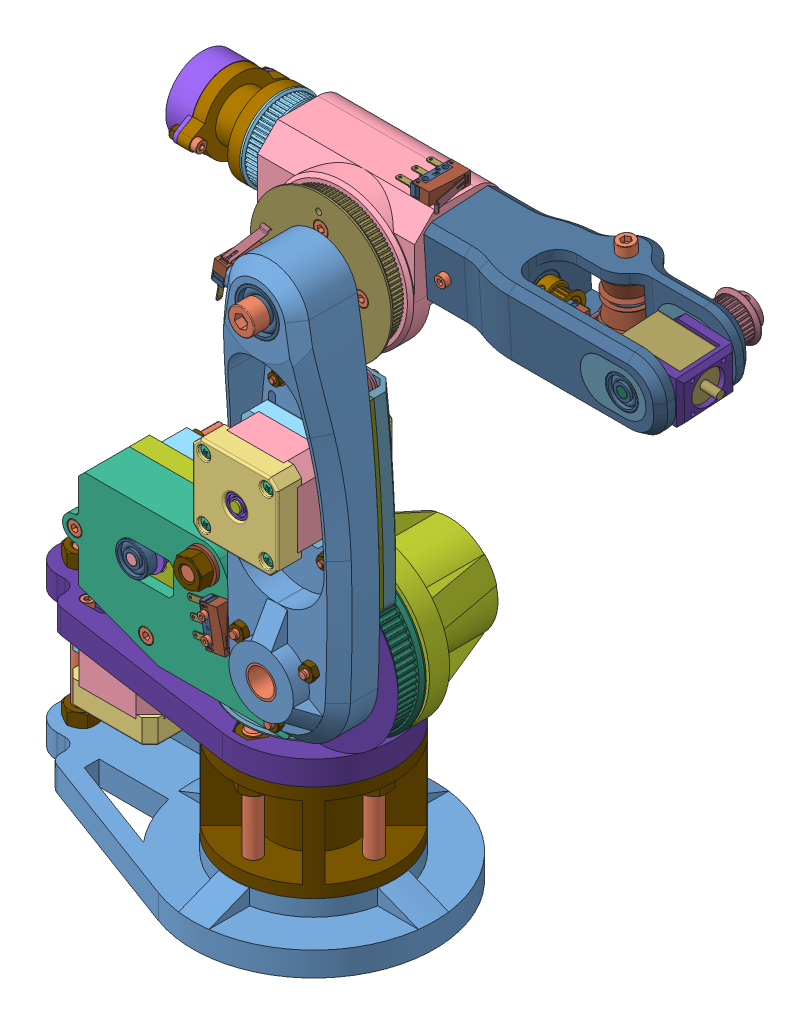
SolidWorks assembly Assem4_v2, configuration Default. Lengths in mm. (continued)
Mates (geometry in assembly coordinates): (continued)
- Coincident20: coincident: plane of Arm1v2-1 through (503.9807 132.9651 88.0417) normal (0 0 -1); plane of socket head cap screw_iso-4 through (159.8987 104.5713 88.0417) normal (0 0 1)
- Coincident21: coincident: plane of GT2_16T_13x14-1 through (144.3987 117.3213 84.5417) normal (0 0 -1); plane of Pulley100Tv5-1 through (144.3987 195.6213 84.5417) normal (0 0 -1)
- Concentric24: concentric: cylinder of socket head cap screw_iso-10 through (117.1825 164.449 125.6976) axis (0 0 -1) radius 1.5; cylinder of ? through (117.1825 164.449 162.4476) axis (0 0 -1) radius 1.5
- Concentric25: concentric: cylinder of socket head cap screw_iso-9 through (141.1825 164.449 125.6976) axis (0 0 -1) radius 1.5; cylinder of ? through (141.1825 164.449 162.4476) axis (0 0 -1) radius 1.5
- Coincident26: coincident: plane of socket head cap screw_iso-9 through (143.356 166.1338 160.4476) normal (0 0 1); plane of ? through (-589.9815 84.1365 160.4476) normal (0 0 -1)
- Coincident27: coincident: plane of socket head cap screw_iso-10 through (119.9295 164.321 160.4476) normal (0 0 1); plane of ? through (-589.9815 84.1365 160.4476) normal (0 0 -1)
- Concentric26: concentric: cylinder of ? through (129.1825 49.449 162.4476) axis (0 0 -1) radius 7.5; cylinder of HTD3M 80T-1 through (129.1825 49.449 108.7344) axis (0 0 1) radius 7.5
- Coincident28: coincident: plane of ? through (-589.9815 84.1365 142.4476) normal (0 0 -1); plane of HTD3M 80T-1
- Concentric27: concentric: cylinder of socket head cap screw_iso-10 through (132.3987 150.6213 39.2917) axis (0 0 -1) radius 1.5; cylinder of Arm 2.3-1 through (132.3987 150.6213 76.0417) axis (0 0 -1) radius 1.5
- Concentric28: concentric: cylinder of socket head cap screw_iso-9 through (156.3987 150.6213 39.2917) axis (0 0 -1) radius 1.5; cylinder of Arm 2.3-1 through (156.3987 150.6213 76.0417) axis (0 0 -1) radius 1.5
- Concentric29: concentric: cylinder of socket head cap screw_iso-9 through (156.3987 150.6213 39.2917) axis (0 0 -1) radius 1.5; cylinder of Arm 4.3-1 through (156.3987 150.6213 86.0417) axis (0 0 1) radius 1.5
- Concentric30: concentric: cylinder of socket head cap screw_iso-10 through (132.3987 150.6213 39.2917) axis (0 0 -1) radius 1.5; cylinder of Arm 4.3-1 through (132.3987 150.6213 86.0417) axis (0 0 1) radius 1.5
- Coincident30: coincident: plane of Arm1v2-1 through (503.9807 132.9651 88.0417) normal (0 0 -1); plane of Arm 4.3-1 through (-574.7652 70.3088 88.0417) normal (0 0 1)
- Coincident31: coincident: plane of plain washer normal grade a_iso-6 through (156.3987 152.2213 86.0417) normal (0 0 1); plane of Arm 4.3-1 through (-574.7652 70.3088 86.0417) normal (0 0 -1)
- Coincident32: coincident: plane of plain washer normal grade a_iso-4 through (132.3987 152.2213 86.0417) normal (0 0 1); plane of Arm 4.3-1 through (-574.7652 70.3088 86.0417) normal (0 0 -1)
- Coincident33: coincident: plane of Arm 2.3-1 through (-574.7652 70.3088 86.0417) normal (0 0 1); plane of Arm 4.3-1 through (-574.7652 70.3088 86.0417) normal (0 0 -1)
- Concentric31: concentric: cylinder of HTD3M 80T-1 through (144.3987 35.6213 107.6549) axis (0 0 -1) radius 7.5; cylinder of HTD80T 2mm spacer-1 through (144.3987 35.6213 65.2285) axis (0 0 1) radius 7.5
- Coincident35: coincident: plane of HTD3M 80T-1 through (144.3987 35.6213 86.4417) normal (0 0 1); plane of HTD80T 2mm spacer-1 through (144.3987 35.6213 86.4417) normal (0 0 -1)
- Concentric32: concentric: cylinder of Arm1v2-1 through (144.3987 195.6213 111.0417) axis (0 0 1) radius 11.1; cylinder of angular contact ball bearing_68_iso-2 through (144.3987 195.6213 135.1792) axis (0 0 -1) radius 11
- Coincident36: coincident: plane of Arm1v2-1 through (144.3987 195.6213 111.0417) normal (0 0 1); plane of angular contact ball bearing_68_iso-2 through (152.8397 202.1971 111.0417) normal (0 0 -1)
- Coincident37: coincident: plane of socket head cap screw_iso-9 through (158.5624 152.3187 74.0417) normal (0 0 1); plane of Arm 2.3-1 through (863.5627 70.3088 74.0417) normal (0 0 -1)
- Coincident38: coincident: plane of socket head cap screw_iso-10 through (135.1322 150.3199 74.0417) normal (0 0 1); plane of Arm 2.3-1 through (863.5627 70.3088 74.0417) normal (0 0 -1)
- Coincident39: coincident: circle of Arm 2.3-1; cylinder of socket head cap screw_iso-11 through (156.3987 83.6213 39.2917) axis (0 0 -1) radius 1.5
- Coincident40: coincident: plane of Arm 2.3-1 through (863.5627 70.3088 74.0417) normal (0 0 -1); plane of socket head cap screw_iso-11 through (158.5624 85.3187 74.0417) normal (0 0 1)
- Concentric33: concentric: cylinder of Arm 2.3-1 through (132.3987 83.6213 80.2843) axis (0 0 -1) radius 1.5; cylinder of socket head cap screw_iso-12 through (132.3987 83.6213 39.2917) axis (0 0 -1) radius 1.5
- Coincident41: coincident: plane of Arm 2.3-1 through (863.5627 70.3088 74.0417) normal (0 0 -1); plane of socket head cap screw_iso-12 through (134.5624 85.3187 74.0417) normal (0 0 1)
- Concentric34: concentric: cylinder of HTD3M 80T-1 through (127.0782 45.6213 92.0986) axis (0 0 -1) radius 2; cylinder of HTD80T 2mm spacer-1 through (127.0782 45.6213 80.7849) axis (0 0 1) radius 2
- Coincident42: coincident: plane of Arm1v2-1 through (503.9807 132.9651 88.0417) normal (0 0 -1); plane of HTD80T 2mm spacer-1 through (144.3987 35.6213 88.0417) normal (0 0 1)
- Concentric35: concentric: cylinder of Arm1v2-1 through (144.3987 35.6213 66.8285) axis (0 0 1) radius 7.5; cylinder of HTD3M 80T-1 through (144.3987 35.6213 107.6549) axis (0 0 -1) radius 7.5
- Concentric36: concentric: cylinder of Arm1v2-1 through (127.0782 45.6213 82.3849) axis (0 0 1) radius 2; cylinder of HTD3M 80T-1 through (127.0782 45.6213 92.0986) axis (0 0 -1) radius 2
- Concentric37: concentric: cylinder of HTD3M 80T-1 through (161.7192 45.6213 92.0986) axis (0 0 -1) radius 2; cylinder of socket head cap screw_iso-14 through (161.7192 45.6213 42.2917) axis (0 0 -1) radius 3.5
- Coincident43: coincident: plane of HTD3M 80T-1 through (161.7192 45.6213 78.0417) normal (0 0 -1); plane of socket head cap screw_iso-14 through (161.7192 49.1213 78.0417) normal (0 0 1)
- Concentric38: concentric: cylinder of HTD3M 80T-1 through (127.0782 45.6213 92.0986) axis (0 0 -1) radius 2; cylinder of socket head cap screw_iso-15 through (127.0782 45.6213 42.2917) axis (0 0 -1) radius 3.5
- Coincident44: coincident: plane of HTD3M 80T-1 through (127.0782 45.6213 78.0417) normal (0 0 -1); plane of socket head cap screw_iso-15 through (127.0782 49.1213 78.0417) normal (0 0 1)
- Concentric39: concentric: cylinder of HTD3M 80T-1 through (144.3987 15.6213 92.0986) axis (0 0 -1) radius 2; cylinder of socket head cap screw_iso-16 through (144.3987 15.6213 42.2917) axis (0 0 -1) radius 3.5
- Coincident45: coincident: plane of HTD3M 80T-1 through (144.3987 15.6213 78.0417) normal (0 0 -1); plane of socket head cap screw_iso-16 through (144.3987 19.1213 78.0417) normal (0 0 1)
- Coincident46: coincident: plane of Arm1v2-1 through (129.1825 49.449 195.2476) normal (0 0 1); plane of ? through (151.6051 52.7817 195.2476) normal (0 0 -1)
- Concentric40: concentric: cylinder of Arm1v2-1 through (146.503 59.449 169.5908) axis (0 0 1) radius 2; cylinder of ? through (146.503 59.449 230.1726) axis (0 0 1) radius 2.15
- Coincident47: coincident: plane of Arm1v2-1 through (129.1825 49.449 195.2476) normal (0 0 1); plane of ? through (146.503 61.599 195.2476) normal (0 0 -1)
- Concentric41: concentric: cylinder of socket head cap screw_iso-14 through (161.7192 45.6213 42.2917) axis (0 0 -1) radius 2; cylinder of hex nut style 1 gradeab_iso-2 through (161.7192 45.6213 133.0792) axis (0 0 -1) radius 2
- Concentric42: concentric: cylinder of socket head cap screw_iso-16 through (144.3987 15.6213 42.2917) axis (0 0 -1) radius 2; cylinder of hex nut style 1 gradeab_iso-3 through (144.3987 15.6213 133.0792) axis (0 0 -1) radius 2
- Concentric43: concentric: cylinder of socket head cap screw_iso-15 through (127.0782 45.6213 42.2917) axis (0 0 -1) radius 2; cylinder of hex nut style 1 gradeab_iso-4 through (127.0782 45.6213 133.0792) axis (0 0 -1) radius 2
- Coincident48: coincident: plane of Arm1v2-1 through (144.3987 35.6213 108.0417) normal (0 0 1); plane of hex nut style 1 gradeab_iso-2 through (159.8824 49.2212 108.0417) normal (0 0 -1)
- Coincident49: coincident: plane of Arm1v2-1 through (144.3987 35.6213 108.0417) normal (0 0 1); plane of hex nut style 1 gradeab_iso-3 through (142.3445 19.1018 108.0417) normal (0 0 -1)
- Coincident50: coincident: plane of Arm1v2-1 through (144.3987 35.6213 108.0417) normal (0 0 1); plane of hex nut style 1 gradeab_iso-4 through (125.5301 49.3545 108.0417) normal (0 0 -1)
- Concentric44: concentric: cylinder of Arm1v2-1 through (132.3987 150.6213 99.2843) axis (0 0 -1) radius 1.5; cylinder of plain washer normal grade a_iso-12 through (132.3987 150.6213 129.9667) axis (0 0 1) radius 1.6
- Coincident51: coincident: plane of Arm1v2-1 through (503.9807 132.9651 95.0417) normal (0 0 1); plane of plain washer normal grade a_iso-12 through (132.3987 152.2213 95.0417) normal (0 0 -1)
- Concentric45: concentric: cylinder of Arm1v2-1 through (156.3987 150.6213 99.2843) axis (0 0 -1) radius 1.5; cylinder of plain washer normal grade a_iso-13 through (156.3987 150.6213 129.9667) axis (0 0 1) radius 1.6
- Coincident52: coincident: plane of Arm1v2-1 through (503.9807 132.9651 95.0417) normal (0 0 1); plane of plain washer normal grade a_iso-13 through (156.3987 152.2213 95.0417) normal (0 0 -1)
- Concentric46: concentric: cylinder of socket head cap screw_iso-12 through (132.3987 83.6213 39.2917) axis (0 0 -1) radius 1.5; cylinder of plain washer normal grade a_iso-14 through (132.3987 83.6213 129.9667) axis (0 0 1) radius 1.6
- Coincident53: coincident: plane of Arm1v2-1 through (503.9807 132.9651 95.0417) normal (0 0 1); plane of plain washer normal grade a_iso-14 through (132.3987 85.2213 95.0417) normal (0 0 -1)
- Concentric47: concentric: cylinder of socket head cap screw_iso-11 through (156.3987 83.6213 39.2917) axis (0 0 -1) radius 1.5; cylinder of plain washer normal grade a_iso-15 through (156.3987 83.6213 129.9667) axis (0 0 1) radius 1.6
- Coincident54: coincident: plane of Arm1v2-1 through (503.9807 132.9651 95.0417) normal (0 0 1); plane of plain washer normal grade a_iso-15 through (156.3987 85.2213 95.0417) normal (0 0 -1)
- Concentric48: concentric: cylinder of socket head cap screw_iso-9 through (156.3987 150.6213 39.2917) axis (0 0 -1) radius 1.5; cylinder of hex nut style 1 gradeab_iso-6 through (156.3987 150.6213 120.5792) axis (0 0 -1) radius 1.5
- Concentric49: concentric: cylinder of socket head cap screw_iso-10 through (132.3987 150.6213 39.2917) axis (0 0 -1) radius 1.5; cylinder of hex nut style 1 gradeab_iso-7 through (132.3987 150.6213 120.5792) axis (0 0 -1) radius 1.5
- Concentric51: concentric: cylinder of socket head cap screw_iso-12 through (132.3987 83.6213 39.2917) axis (0 0 -1) radius 1.5; cylinder of hex nut style 1 gradeab_iso-8 through (132.3987 83.6213 97.9417) axis (0 0 -1) radius 1.25
- Coincident55: coincident: plane of plain washer normal grade a_iso-14 through (132.3987 87.1213 95.5417) normal (0 0 1); plane of hex nut style 1 gradeab_iso-8 through (129.9384 85.6288 95.5417) normal (0 0 -1)
- Concentric53: concentric: cylinder of socket head cap screw_iso-11 through (141.1825 97.449 126.4976) axis (0 0 -1) radius 1.5; cylinder of ? through (141.1825 97.449 159.6101) axis (0 0 1) radius 1.5
- Coincident57: coincident: plane of plain washer normal grade a_iso-15 through (156.3987 87.1213 95.5417) normal (0 0 1); plane of hex nut style 1 gradeab_iso-11 through (153.9384 85.6288 95.5417) normal (0 0 -1)
- Concentric54: concentric: cylinder of socket head cap screw_iso-11 through (156.3987 83.6213 39.2917) axis (0 0 -1) radius 1.5; cylinder of hex nut style 1 gradeab_iso-11 through (156.3987 83.6213 97.9417) axis (0 0 -1) radius 1.25
- Coincident58: coincident: plane of plain washer normal grade a_iso-12 through (132.3987 154.1213 95.5417) normal (0 0 1); plane of hex nut style 1 gradeab_iso-7 through (131.3661 153.6242 95.5417) normal (0 0 -1)
- Coincident59: coincident: plane of plain washer normal grade a_iso-13 through (156.3987 154.1213 95.5417) normal (0 0 1); plane of hex nut style 1 gradeab_iso-6 through (155.3038 153.602 95.5417) normal (0 0 -1)
- Concentric55: concentric: cylinder of socket head cap screw_iso-7 through (144.3987 248.3713 157.3917) axis (0 0 1) radius 4; cylinder of ? through (144.3987 248.3713 25.128) axis (0 0 1) radius 4
- Coincident60: coincident: plane of Pulley100Tv5-1 through (144.3987 248.3713 76.4417) normal (0 0 -1); plane of ? through (144.3987 248.3713 76.4417) normal (0 0 1)
- Concentric56: concentric: cylinder of ? through (118.6992 268.756 55.4417) axis (-0.999889 0.014881 0) radius 16; cylinder of angular contact ball bearing_68_iso-4 through (93.5645 269.1301 55.4417) axis (0.999889 -0.014881 0) radius 16
- Coincident61: coincident: plane of ? through (118.6992 268.756 55.4417) normal (-0.999889 0.014881 0); plane of angular contact ball bearing_68_iso-4
- Concentric57: concentric: cylinder of ? through (170.6935 267.9822 55.4417) axis (0.999889 -0.014881 0) radius 16; cylinder of angular contact ball bearing_68_iso-3 through (154.5578 268.2223 55.4417) axis (0.999889 -0.014881 0) radius 16
- Coincident62: coincident: plane of ? through (170.6935 267.9822 55.4417) normal (0.999889 -0.014881 0); plane of angular contact ball bearing_68_iso-3
- Concentric58: concentric: cylinder of angular contact ball bearing_68_iso-3 through (154.2612 210.6213 52.4417) axis (1 0 0) radius 7.5; cylinder of 100mm aluputki-1 through (211.1987 210.6213 52.4417) axis (-1 0 0) radius 7.5
- Concentric59: concentric: cylinder of angular contact ball bearing_68_iso-4 through (85.2612 210.6213 52.4417) axis (1 0 0) radius 7.5; cylinder of 100mm aluputki-1 through (211.1987 210.6213 52.4417) axis (-1 0 0) radius 7.5
- Concentric60: concentric: cylinder of HTD3M 80T-1 through (144.3987 35.6213 107.6549) axis (0 0 -1) radius 7.5; cylinder of 90mm aluputki-1 through (144.3987 35.6213 116.0417) axis (0 0 -1) radius 7.5
- Coincident63: coincident: plane of Arm1v2-1 through (144.3987 35.6213 116.0417) normal (0 0 1); plane of 90mm aluputki-1 through (144.3987 35.6213 116.0417) normal (0 0 1)
- Concentric61: concentric: cylinder of 90mm aluputki-1 through (144.3987 35.6213 116.0417) axis (0 0 -1) radius 7.5; cylinder of angular contact ball bearing_68_iso-5 through (144.3987 35.6213 47.3042) axis (0 0 1) radius 7.5
- Concentric62: concentric: cylinder of 90mm aluputki-1 through (144.3987 35.6213 116.0417) axis (0 0 -1) radius 7.5; cylinder of angular contact ball bearing_68_iso-6 through (144.3987 35.6213 6.3042) axis (0 0 1) radius 7.5
- Concentric63: concentric: cylinder of 90mm aluputki-1 through (144.3987 35.6213 116.0417) axis (0 0 -1) radius 7.5; cylinder of 15mm 1.6 rikka-1 through (144.3987 35.6213 72.4417) axis (0 0 1) radius 7.5
- Coincident64: coincident: plane of HTD3M 80T-1 through (144.3987 35.6213 74.0417) normal (0 0 -1); plane of 15mm 1.6 rikka-1 through (144.3987 35.6213 74.0417) normal (0 0 1)
- Coincident65: coincident: plane of angular contact ball bearing_68_iso-5 through (148.8906 41.9981 72.4417) normal (0 0 1); plane of 15mm 1.6 rikka-1 through (144.3987 35.6213 72.4417) normal (0 0 -1)
- Concentric76: concentric: cylinder of ? through (96.8987 103.3713 77.4417) axis (0 0 1) radius 11.2; cylinder of angular contact ball bearing_68_iso-7 through (96.8987 103.3713 101.5792) axis (0 0 -1) radius 11
- Coincident76: coincident: plane of ? through (96.8987 103.3713 77.4417) normal (0 0 1); plane of angular contact ball bearing_68_iso-7 through (96.8987 114.0713 77.4417) normal (0 0 -1)
- Concentric77: concentric: cylinder of socket head cap screw_iso-23 through (94.3987 50.6213 22.6917) axis (0 0 -1) radius 4; cylinder of angular contact ball bearing_68_iso-7 through (94.3987 50.6213 98.1792) axis (0 0 -1) radius 4
- Concentric78: concentric: cylinder of socket head cap screw_iso-23 through (96.8987 103.3713 22.6917) axis (0 0 -1) radius 4; cylinder of ? through (96.8987 103.3713 72.4417) axis (0 0 1) radius 4
- Coincident78: coincident: plane of angular contact ball bearing_68_iso-7 through (96.8987 107.6713 77.4417) normal (0 0 -1); plane of ? through (96.8987 103.3713 77.4417) normal (0 0 1)
- Concentric79: concentric: cylinder of socket head cap screw_iso-7 through (144.3987 195.6213 157.7917) axis (0 0 1) radius 4; cylinder of Arm2Mountv2-1 through (144.3987 195.6213 74.8417) axis (0 0 1) radius 4
- Coincident79: coincident: plane of Pulley100Tv5-1 through (144.3987 195.6213 76.8417) normal (0 0 -1); plane of Arm2Mountv2-1 through (144.3987 195.6213 76.8417) normal (0 0 1)
- Concentric80: concentric: cylinder of angular contact ball bearing_68_iso-3 through (154.2612 210.6213 52.4417) axis (1 0 0) radius 16; cylinder of Arm2Mountv2-1 through (170.3987 210.6213 52.4417) axis (1 0 0) radius 16.25
- Coincident80: coincident: plane of angular contact ball bearing_68_iso-3 through (170.3987 213.691 66.3828) normal (-1 0 0); plane of Arm2Mountv2-1 through (170.3987 210.6213 52.4417) normal (1 0 0)
- Concentric81: concentric: cylinder of angular contact ball bearing_68_iso-4 through (85.2612 210.6213 52.4417) axis (1 0 0) radius 16; cylinder of Arm2Mountv2-1 through (110.3987 210.6213 52.4417) axis (-1 0 0) radius 16.25
- Coincident81: coincident: plane of angular contact ball bearing_68_iso-4 through (110.3987 196.3072 58.8913) normal (1 0 0); plane of Arm2Mountv2-1 through (110.3987 210.6213 52.4417) normal (-1 0 0)
- Concentric82: concentric: cylinder of 100mm aluputki-1 through (211.1987 210.6213 52.4417) axis (-1 0 0) radius 7.5; cylinder of Pulley60Tv2-1 through (100.1987 210.6213 52.4417) axis (1 0 0) radius 7.5
- Concentric83: concentric: cylinder of 100mm aluputki-1 through (242.6976 267.2683 56.4417) axis (-0.998565 -0.053553 0) radius 7.5; cylinder of ? through (121.2721 260.7562 56.4417) axis (0.998565 0.053553 0) radius 7.75
- Coincident83: coincident: plane of angular contact ball bearing_68_iso-4; plane of ? through (122.8698 260.8419 56.4417) normal (0.998565 0.053553 0)
- Coincident84: coincident: plane of Pulley60Tv2-1; plane of ? through (121.2721 260.7562 56.4417) normal (-0.998565 -0.053553 0)
- Concentric84: concentric: cylinder of Arm2Mountv2-1 through (116.8408 282.6024 18.0417) axis (0.998699 0.050996 0) radius 1.75; cylinder of ? through (87.0793 281.0828 18.0417) axis (-0.998699 -0.050996 0) radius 2.75
- Coincident85: coincident: plane of Arm2Mountv2-1; plane of ? through (121.644 285.5995 18.1414) normal (0.998699 0.050996 0)
- Concentric85: concentric: cylinder of Arm2Mountv2-1 through (119.0795 238.7596 18.0417) axis (0.998699 0.050996 0) radius 1.75; cylinder of ? through (89.318 237.2399 18.0417) axis (-0.998699 -0.050996 0) radius 2.75
- Coincident86: coincident: plane of Arm2Mountv2-1; plane of ? through (123.8826 241.7583 18.021) normal (0.998699 0.050996 0)
- Concentric86: concentric: cylinder of ? through (129.7737 283.2628 18.0417) axis (-0.998699 -0.050996 0) radius 1.75; cylinder of ? through (87.0793 281.0828 18.0417) axis (-0.998699 -0.050996 0) radius 1.5
- Concentric87: concentric: cylinder of ? through (132.0124 239.4199 18.0417) axis (-0.998699 -0.050996 0) radius 1.75; cylinder of ? through (89.318 237.2399 18.0417) axis (-0.998699 -0.050996 0) radius 1.5
- Coincident87: coincident: plane of Arm2Mountv2-1; plane of ? through (128.8957 261.2394 18.0417) normal (-0.998699 -0.050996 0)
- Concentric88: concentric: cylinder of ? through (87.0793 281.0828 18.0417) axis (-0.998699 -0.050996 0) radius 1.5; cylinder of ? through (132.1706 283.3852 18.0417) axis (-0.998699 -0.050996 0) radius 1.25
- Coincident88: coincident: plane of ? through (129.7737 283.2628 18.0417) normal (0.998699 0.050996 0); plane of ? through (129.6147 286.3774 18.6397) normal (-0.998699 -0.050996 0)
- Concentric89: concentric: cylinder of ? through (89.318 237.2399 18.0417) axis (-0.998699 -0.050996 0) radius 1.5; cylinder of ? through (134.4093 239.5423 18.0417) axis (-0.998699 -0.050996 0) radius 1.25
- Coincident89: coincident: plane of ? through (132.0124 239.4199 18.0417) normal (0.998699 0.050996 0); plane of ? through (131.9075 241.4753 15.6234) normal (-0.998699 -0.050996 0)
- Concentric90: concentric: cylinder of ? through (121.4054 260.8569 18.0417) axis (0.998699 0.050996 0) radius 2.5; cylinder of GT2_16T_13x14-2 through (126.3989 261.1119 18.0417) axis (-0.998699 -0.050996 0) radius 2.5
- Distance2: distance = 0.5 mm: plane of ? through (126.8983 261.1374 18.0417) normal (-0.998699 -0.050996 0); plane of GT2_16T_13x14-2
- Concentric91: concentric: cylinder of 100mm aluputki-1 through (211.1987 210.6213 52.4417) axis (-1 0 0) radius 7.5; cylinder of 15mm rikka 1.2mm-1 through (100.1987 210.6213 52.4417) axis (1 0 0) radius 7.5
- Coincident91: coincident: plane of angular contact ball bearing_68_iso-4 through (101.3987 201.4585 56.5702) normal (-1 0 0); plane of 15mm rikka 1.2mm-1 through (101.3987 210.6213 52.4417) normal (1 0 0)
- Coincident92: coincident: plane of Pulley60Tv2-1 through (100.1987 224.518 40.5133) normal (1 0 0); plane of 15mm rikka 1.2mm-1 through (100.1987 210.6213 52.4417) normal (-1 0 0)
- Concentric97: concentric: cylinder of Nema 14 stepper-1 through (119.2243 236.5858 35.8417) axis (-0.99443 0.105397 0) radius 1.5; cylinder of ? through (72.2375 241.5658 35.8417) axis (-0.99443 0.105397 0) radius 1.5
- Concentric98: concentric: cylinder of Nema 14 stepper-1 through (116.484 210.7307 61.8417) axis (-0.99443 0.105397 0) radius 1.5; cylinder of ? through (69.4971 215.7106 61.8417) axis (-0.99443 0.105397 0) radius 1.5
- Coincident98: coincident: plane of Pulley60Tv2-1 through (98.6987 210.6213 52.4417) normal (-1 0 0); plane of GT2_16T_13x14-2 through (98.6987 168.7922 48.8417) normal (-1 0 0)
- Concentric100: concentric: cylinder of 100mm aluputki-1 through (211.1987 210.6213 52.4417) axis (-1 0 0) radius 7.5; cylinder of Motor 5 adapter-1 through (84.1987 210.6213 52.4417) axis (1 0 0) radius 7.5
- Coincident99: coincident: plane of Pulley60Tv2-1 through (90.1987 225.7973 39.4152) normal (-1 0 0); plane of Motor 5 adapter-1 through (90.1987 210.6213 52.4417) normal (1 0 0)
- Coincident101: coincident: plane of 100mm aluputki-1 through (66.1987 210.6213 52.4417) normal (-1 0 0); plane of Motor 5 adapter-1 through (66.1987 210.6213 52.4417) normal (-1 0 0)
- Concentric102: concentric: cylinder of Nema 14 Round stepper-2 through (62.1987 209.2012 74.3457) axis (1 0 0) radius 1.75; cylinder of Motor 5 adapter-1 through (84.7778 209.2012 74.3457) axis (-1 0 0) radius 1.75
- Concentric103: concentric: cylinder of Nema 14 Round stepper-2 through (62.1987 212.0414 30.5377) axis (1 0 0) radius 1.75; cylinder of Motor 5 adapter-1 through (84.7778 212.0414 30.5377) axis (-1 0 0) radius 1.75
- Coincident102: coincident: plane of Nema 14 Round stepper-2 through (64.1987 210.6213 52.4417) normal (1 0 0); plane of Motor 5 adapter-1 through (64.1987 210.6213 52.4417) normal (-1 0 0)
- Concentric104: concentric: cylinder of Motor 5 adapter-1 through (84.7778 209.2012 74.3457) axis (-1 0 0) radius 1.75; cylinder of socket head cap screw_iso-33 through (104.9487 209.2012 74.3457) axis (1 0 0) radius 2.75
- Coincident103: coincident: plane of Motor 5 adapter-1 through (70.1987 210.6213 52.4417) normal (1 0 0); plane of socket head cap screw_iso-33 through (70.1987 206.5205 73.7322) normal (-1 0 0)
- Concentric105: concentric: cylinder of Motor 5 adapter-1 through (84.7778 212.0414 30.5377) axis (-1 0 0) radius 1.75; cylinder of socket head cap screw_iso-34 through (104.9487 212.0414 30.5377) axis (1 0 0) radius 2.75
- Coincident104: coincident: plane of Motor 5 adapter-1 through (70.1987 210.6213 52.4417) normal (1 0 0); plane of socket head cap screw_iso-34 through (70.1987 211.8181 27.7968) normal (-1 0 0)
- Concentric106: concentric: cylinder of socket head cap screw_iso-33 through (104.9487 209.2012 74.3457) axis (1 0 0) radius 1.5; cylinder of hex nut style 1 gradeab_iso-16 through (59.7987 209.2012 74.3457) axis (1 0 0) radius 1.25
- Coincident105: coincident: plane of Nema 14 Round stepper-2 through (62.1987 209.2012 74.3457) normal (-1 0 0); plane of hex nut style 1 gradeab_iso-16 through (62.1987 209.9536 71.2607) normal (1 0 0)
- Concentric107: concentric: cylinder of socket head cap screw_iso-34 through (104.9487 212.0414 30.5377) axis (1 0 0) radius 1.5; cylinder of hex nut style 1 gradeab_iso-15 through (59.7987 212.0414 30.5377) axis (1 0 0) radius 1.25
- Coincident106: coincident: plane of Nema 14 Round stepper-2 through (62.1987 212.0414 30.5377) normal (-1 0 0); plane of hex nut style 1 gradeab_iso-15 through (62.1987 213.4668 27.7002) normal (1 0 0)
- Concentric109: concentric: cylinder of socket head cap screw_iso-23 through (94.3987 50.6213 22.6917) axis (0 0 -1) radius 4; cylinder of plain washer normal grade a_iso-18 through (94.3987 50.6213 54.7167) axis (0 0 -1) radius 4.2
- Concentric110: concentric: cylinder of socket head cap screw_iso-23 through (94.3987 50.6213 22.6917) axis (0 0 -1) radius 4; cylinder of angular contact ball bearing_68_iso-8 through (94.3987 50.6213 105.1792) axis (0 0 -1) radius 4
- Coincident108: coincident: plane of angular contact ball bearing_68_iso-7 through (92.8966 54.6504 74.0417) normal (0 0 -1); plane of plain washer normal grade a_iso-17 through (94.3987 58.6213 74.0417) normal (0 0 1)
- Coincident109: coincident: plane of angular contact ball bearing_68_iso-7 through (92.2678 56.337 81.0417) normal (0 0 1); plane of angular contact ball bearing_68_iso-8 through (93.9304 54.8957 81.0417) normal (0 0 -1)
- Coincident110: coincident: plane of plain washer normal grade a_iso-18 through (94.3987 58.6213 88.0417) normal (0 0 -1); plane of angular contact ball bearing_68_iso-8 through (93.7344 56.685 88.0417) normal (0 0 1)
- Concentric112: concentric: cylinder of socket head cap screw_iso-23 through (94.3987 50.6213 22.6917) axis (0 0 -1) radius 4; cylinder of hex nut style 1 gradeab_iso-18 through (94.3987 50.6213 103.0417) axis (0 0 -1) radius 3.4
- Coincident115: coincident: plane of plain washer normal grade a_iso-20 through (87.6357 54.8946 96.2417) normal (0 0 1); plane of hex nut style 1 gradeab_iso-18 through (96.0657 57.9394 96.2417) normal (0 0 -1)
- Concentric113: concentric: cylinder of Microswitch-SS-3GL13SL-1/limit-switch-bottomcase-1 through (101.319 35.6213 100.8417) axis (0 0 -1) radius 1.25; cylinder of socket head cap screw_iso-36 through (101.319 35.6213 134.5917) axis (0 0 1) radius 1.9
- Coincident116: coincident: plane of ? through (102.8008 37.5834 100.8417) normal (0 0 1); plane of socket head cap screw_iso-36 through (101.319 37.5213 100.8417) normal (0 0 -1)
- Concentric114: concentric: cylinder of ? through (103.0555 25.7732 100.8417) axis (0 0 -1) radius 1.25; cylinder of socket head cap screw_iso-37 through (103.0555 25.7732 134.5917) axis (0 0 1) radius 1.9
- Coincident117: coincident: plane of ? through (102.8008 37.5834 100.8417) normal (0 0 1); plane of socket head cap screw_iso-37 through (103.0555 27.6732 100.8417) normal (0 0 -1)
- Concentric117: concentric: cylinder of Nema 14 stepper-1 through (119.2243 236.5858 61.8417) axis (-0.99443 0.105397 0) radius 1.5; cylinder of ? through (72.2375 241.5658 61.8417) axis (-0.99443 0.105397 0) radius 1.5
- Concentric118: concentric: cylinder of Nema 14 stepper-1 through (116.484 210.7307 35.8417) axis (-0.99443 0.105397 0) radius 1.5; cylinder of ? through (69.4971 215.7106 35.8417) axis (-0.99443 0.105397 0) radius 1.5
- Coincident119: coincident: plane of Arm2Mountv2-1; plane of ? through (106.8409 238.3467 33.1281) normal (0.99443 -0.105397 0)
- Coincident120: coincident: plane of Arm2Mountv2-1; plane of ? through (107.0666 240.4761 60.9097) normal (0.99443 -0.105397 0)
- Coincident121: coincident: plane of Arm2Mountv2-1; plane of ? through (104.3434 214.7828 35.842) normal (0.99443 -0.105397 0)
- Coincident122: coincident: plane of Arm2Mountv2-1; plane of ? through (104.3434 214.7825 61.8047) normal (0.99443 -0.105397 0)
- Concentric121: concentric: cylinder of Arm2Mountv2-1 through (126.7032 235.7932 35.8417) axis (-0.99443 0.105397 0) radius 1.75; cylinder of ? through (72.2375 241.5658 35.8417) axis (-0.99443 0.105397 0) radius 1.5
- Concentric122: concentric: cylinder of Arm2Mountv2-1 through (126.7032 235.7932 61.8417) axis (-0.99443 0.105397 0) radius 1.75; cylinder of ? through (72.2375 241.5658 61.8417) axis (-0.99443 0.105397 0) radius 1.5
- Concentric123: concentric: cylinder of Arm2Mountv2-1 through (104.3987 181.7922 35.8417) axis (-1 0 0) radius 3; cylinder of socket head cap screw_iso-39 through (69.6487 181.7922 35.8417) axis (-1 0 0) radius 2.75
- Coincident124: coincident: plane of Arm2Mountv2-1 through (104.3987 189.7922 35.8417) normal (-1 0 0); plane of socket head cap screw_iso-39 through (104.3987 184.3472 36.8589) normal (1 0 0)
- Concentric124: concentric: cylinder of Arm2Mountv2-1 through (104.3987 181.7922 61.8417) axis (-1 0 0) radius 3; cylinder of socket head cap screw_iso-40 through (69.6487 181.7922 61.8417) axis (-1 0 0) radius 2.75
- Coincident125: coincident: plane of Arm2Mountv2-1 through (104.3987 189.7922 61.8417) normal (-1 0 0); plane of socket head cap screw_iso-40 through (104.3987 184.3472 62.8589) normal (1 0 0)
- Concentric125: concentric: cylinder of Arm2Mountv2-1 through (104.3987 155.7922 61.8417) axis (-1 0 0) radius 3; cylinder of socket head cap screw_iso-41 through (69.6487 155.7922 61.8417) axis (-1 0 0) radius 2.75
- Coincident126: coincident: plane of Arm2Mountv2-1 through (104.3987 163.7922 61.8417) normal (-1 0 0); plane of socket head cap screw_iso-41 through (104.3987 158.3472 62.8589) normal (1 0 0)
- Coincident127: coincident: plane of Arm2Mountv2-1 through (104.3987 163.7922 35.8417) normal (-1 0 0); plane of socket head cap screw_iso-42 through (104.3987 158.5349 35.6417) normal (1 0 0)
- Concentric127: concentric: cylinder of Nema 14 stepper-1 through (113.8987 181.7922 35.8417) axis (-1 0 0) radius 1.5; cylinder of socket head cap screw_iso-39 through (69.6487 181.7922 35.8417) axis (-1 0 0) radius 1.5
- Concentric128: concentric: cylinder of Nema 14 stepper-1 through (113.8987 155.7922 61.8417) axis (-1 0 0) radius 1.5; cylinder of socket head cap screw_iso-41 through (69.6487 155.7922 61.8417) axis (-1 0 0) radius 1.5
- Concentric130: concentric: cylinder of Pulley100Tv5-1 through (144.3987 215.6213 70.6192) axis (0 0 1) radius 2.2; cylinder of Arm2Mountv2-1 through (144.3987 215.6213 64.8417) axis (0 0 1) radius 2
- Coincident128: coincident: plane of Pulley100Tv5-1 through (155.4871 247.9866 86.4417) normal (0 0 1); plane of ? through (126.3632 254.9408 86.4417) normal (0 0 -1)
- Concentric131: concentric: cylinder of Pulley100Tv5-1 through (144.3987 215.6213 70.6192) axis (0 0 1) radius 2.2; cylinder of socket head cap screw_iso-44 through (144.3987 215.6213 118.1917) axis (0 0 1) radius 3.5
- Coincident129: coincident: plane of Pulley100Tv5-1 through (144.3987 215.6213 82.4417) normal (0 0 1); plane of socket head cap screw_iso-44 through (144.3987 219.1213 82.4417) normal (0 0 -1)
- Concentric132: concentric: cylinder of Pulley100Tv5-1 through (164.3987 195.6213 70.6192) axis (0 0 1) radius 2.2; cylinder of socket head cap screw_iso-46 through (164.3987 195.6213 118.1917) axis (0 0 1) radius 3.5
- Coincident130: coincident: plane of Pulley100Tv5-1 through (164.3987 195.6213 82.4417) normal (0 0 1); plane of socket head cap screw_iso-46 through (164.3987 199.1213 82.4417) normal (0 0 -1)
- Concentric133: concentric: cylinder of Pulley100Tv5-1 through (144.3987 175.6213 70.6192) axis (0 0 1) radius 2.2; cylinder of socket head cap screw_iso-47 through (144.3987 175.6213 118.1917) axis (0 0 1) radius 3.5
- Coincident131: coincident: plane of Pulley100Tv5-1 through (144.3987 175.6213 82.4417) normal (0 0 1); plane of socket head cap screw_iso-47 through (144.3987 179.1213 82.4417) normal (0 0 -1)
- Concentric134: concentric: cylinder of Pulley100Tv5-1 through (124.3987 195.6213 70.6192) axis (0 0 1) radius 2.2; cylinder of socket head cap screw_iso-48 through (124.3987 195.6213 118.1917) axis (0 0 1) radius 2
- Coincident133: coincident: plane of Pulley100Tv5-1 through (124.3987 195.6213 82.4417) normal (0 0 1); plane of socket head cap screw_iso-48 through (122.33 198.4445 82.4417) normal (0 0 -1)
- Concentric135: concentric: cylinder of socket head cap screw_iso-7 through (144.3987 195.6213 157.7917) axis (0 0 1) radius 4; cylinder of hex nut style 1 gradeab_iso-19 through (144.3987 195.6213 39.0417) axis (0 0 1) radius 3.4
- Coincident135: coincident: plane of Arm2Mountv2-1 through (144.3987 195.6213 45.8417) normal (0 0 -1); plane of hex nut style 1 gradeab_iso-19 through (148.1515 202.1213 45.8417) normal (0 0 1)
- Parallel3: parallel: plane of Arm2Mountv2-1 through (140.5882 202.2213 45.8417) normal (0 -1 0); plane of hex nut style 1 gradeab_iso-19 through (148.1515 202.1213 39.0417) normal (0 1 0)
- Concentric139: concentric: cylinder of Arm1v2-1 through (126.3636 191.1509 105.5417) axis (-0.985156 0.171661 0) radius 1; cylinder of ? through (114.3447 193.2451 105.5417) axis (0.985156 -0.171661 0) radius 1.25
- Concentric140: concentric: cylinder of Arm1v2-1 through (126.3636 191.1509 95.5417) axis (-0.985156 0.171661 0) radius 1; cylinder of ? through (114.3447 193.2451 95.5417) axis (0.985156 -0.171661 0) radius 1.25
- Coincident139: coincident: plane of Arm1v2-1 through (121.7401 199.5695 110.5417) normal (-0.985156 0.171661 0); plane of Microswitch-SS-3GL13SL-2/limit-switch-top-case-1 through (120.6553 193.3439 98.757) normal (0.985156 -0.171661 0)
- Concentric144: concentric: cone of socket head cap screw_iso-50 through (65.8987 5.6213 55.6417) axis (0 0 -1); cylinder of hex nut style 1 gradeab_iso-21 through (65.8987 5.6213 37.4042) axis (0 0 1) radius 2
- Concentric146: concentric: cylinder of GT2_16T_13x14-2 through (104.8687 168.7922 48.8417) axis (-1 0 0) radius 2.5; cylinder of Nema 14 stepper-1 through (96.8987 168.7922 48.8417) axis (1 0 0) radius 2.5
- Coincident144: coincident: plane of Arm2Mountv2-1 through (109.3987 195.6213 76.8417) normal (1 0 0); plane of Nema 14 stepper-1 through (109.3987 168.7922 48.8417) normal (-1 0 0)
- Concentric152: concentric: cylinder of socket head cap screw_iso-54 through (30.3987 34.1213 126.3917) axis (0 0 1) radius 2; cylinder of hex nut style 1 gradeab_iso-22 through (30.3987 34.1213 64.2417) axis (0 0 1) radius 1.65
- Concentric157: concentric: cylinder of thrust ball bearing_68_iso-1 through (106.8987 -52.6037 52.4417) axis (0 1 0) radius 10; cylinder of thrust ball bearing_68_iso-2 through (106.8987 -46.7537 52.4417) axis (0 -1 0) radius 10
- Coincident158: coincident: plane of Pulley100TBase-2 through (106.8987 -6.3787 52.4417) normal (0 1 0); plane of Bottom spacer-1 through (106.8987 -6.3787 52.4417) normal (0 -1 0); plane of Baseplate-1; plane of assembly
- Parallel5: parallel: plane of Baseplate-1 through (1.8987 -19.6787 77.4417) normal (-1 0 0); plane of assembly through (0 0 0) normal (1 0 0)
- Concentric160: concentric: cylinder of Baseplate-1 through (106.8987 -31.6787 52.4417) axis (0 1 0) radius 16; cylinder of Bottom Tube-1 through (106.8987 -37.6787 52.4417) axis (0 1 0) radius 12.5
- Concentric161: concentric: cylinder of Baseplate-1 through (136.8987 -42.9924 52.4417) axis (0 1 0) radius 4; cylinder of Bottom Tube-1 through (136.8987 -90.9924 52.4417) axis (0 -1 0) radius 4
- Coincident162: coincident: plane of Baseplate-1 through (106.8987 -31.6787 52.4417) normal (0 -1 0); plane of Bottom Tube-1 through (106.8987 -31.6787 52.4417) normal (0 1 0)
- Coincident164: coincident: plane of Bottom Tube-1 through (106.8987 -31.6787 52.4417) normal (0 1 0); plane of angular contact ball bearing_68_iso-9 through (122.5987 -31.6787 52.4417) normal (0 -1 0)
- Concentric163: concentric: cylinder of Baseplate-1 through (106.8987 -31.6787 52.4417) axis (0 1 0) radius 16; cylinder of angular contact ball bearing_68_iso-9 through (106.8987 -6.5412 52.4417) axis (0 -1 0) radius 16
- Coincident165: coincident: plane of thrust ball bearing_68_iso-1 through (106.6815 -22.6787 62.7394) normal (0 -1 0); plane of Baseplate-1 through (106.8987 -22.6787 52.4417) normal (0 1 0)
- Concentric164: concentric: cylinder of Bottom Tube-1 through (106.8987 -37.6787 52.4417) axis (0 1 0) radius 12.5; cylinder of angular contact ball bearing_68_iso-10 through (106.8987 -51.5412 52.4417) axis (0 -1 0) radius 7.5
- Coincident168: coincident: plane of Bottom Tube-1 through (106.8987 -67.6787 52.4417) normal (0 -1 0); plane of angular contact ball bearing_68_iso-10 through (121.1731 -67.6787 52.3049) normal (0 1 0)
- Coincident169: coincident: plane of thrust ball bearing_68_iso-2 through (96.6228 -76.6787 53.1462) normal (0 1 0); plane of Bottom Tube-1 through (106.8987 -76.6787 52.4417) normal (0 -1 0)
- Concentric165: concentric: cylinder of Bottom Tube-1 through (106.8987 -37.6787 52.4417) axis (0 1 0) radius 12.5; cylinder of Bottom support-1 through (106.8987 -79.6787 52.4417) axis (0 -1 0) radius 20
- Concentric168: concentric: cylinder of Pulley100TBase-2 through (131.8987 -0.1561 52.4417) axis (0 -1 0) radius 2.2; cylinder of socket head cap screw_iso-58 through (131.8987 -47.4287 52.4417) axis (0 -1 0) radius 2
- Coincident173: coincident: plane of Pulley100TBase-2 through (131.8987 -11.6787 52.4417) normal (0 -1 0); plane of socket head cap screw_iso-58 through (128.3987 -11.6787 52.4417) normal (0 1 0)
- Concentric169: concentric: cylinder of socket head cap screw_iso-58 through (131.8987 -47.4287 52.4417) axis (0 -1 0) radius 2; cylinder of hex nut style 1 gradeab_iso-24 through (131.8987 8.8213 52.4417) axis (0 -1 0) radius 1.65
- Coincident176: coincident: plane of Bottom Tube-1 through (106.8987 -79.6787 52.4417) normal (0 -1 0); plane of Bottom support-1 through (106.8987 -79.6787 52.4417) normal (0 1 0)
- Concentric170: concentric: cylinder of Bottom Tube-1 through (106.8987 -90.9924 22.4417) axis (0 -1 0) radius 4; cylinder of Bottom support-1 through (106.8987 -110.9924 22.4417) axis (0 1 0) radius 4
